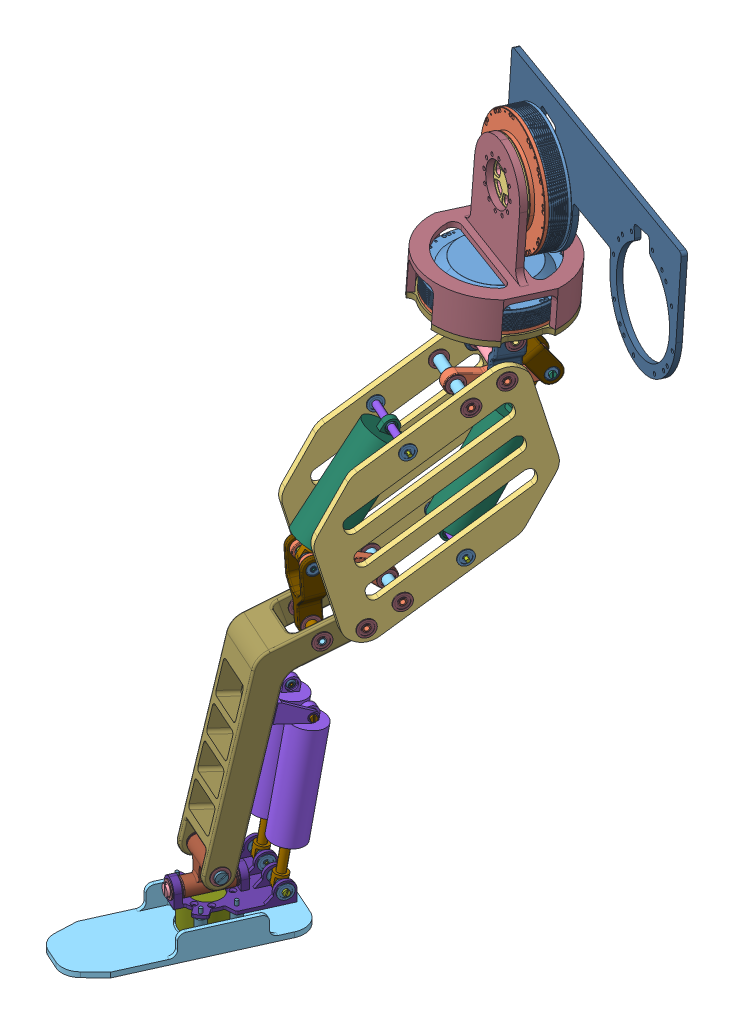
SolidWorks assembly 腿部总装, configuration 默认. Lengths in mm.
Overall size (628.66 1050.26 646.32).
180 component instances, 46 part files, 283 mates.
Components (placement in the parent):
- B1电机模型-220923.STEP-1: B1电机模型-220923.STEP [默认] at (664.8919 713.7763 -8377.8615) x (0.025023 0.998139 -0.055612) z (-0.344283 0.060831 0.936893) size (57.67 170.5 170.5)
  - B1________-220923.STEP.STEP-1: B1________-220923.STEP.STEP [默认] at origin size (57.67 170.5 170.5)
    - 11UXMR1_DVUR40_BCVR1_BASR1.STEP.STEP-1: 11UXMR1_DVUR40_BCVR1_BASR1.STEP.STEP [默认] at (17.5155 -7.1917 170.5) size (43.17 170.5 170.5)
    - 11UXMR1_DVUR40_HOSR1_BASR1.STEP.STEP-1: 11UXMR1_DVUR40_HOSR1_BASR1.STEP.STEP [默认] at (17.5155 -7.1917 170.5) size (28.4 170.5 170.5)
    - 11UXMR1_DVUR40_RDCR1_HLDR1_BHDR1.STEP.STEP-1: 11UXMR1_DVUR40_RDCR1_HLDR1_BHDR1.STEP.STEP [默认] at (17.5155 -7.1917 170.5) x (1 0 0) z (0 0.585761 -0.810484) size (4.4 117.7 117.7)
    - 11UXMR1_DVUR40_RDCR1_HLDR1_BASR1.STEP.STEP-1: 11UXMR1_DVUR40_RDCR1_HLDR1_BASR1.STEP.STEP [默认] at (17.5155 -7.1917 170.5) x (1 0 0) z (0 0.409019 0.912526) size (11.2 84 84)
- 脚掌-1: 脚掌 [默认] at (397.9595 0 -7737.8464) x (0.410325 0 -0.911939) z (0.911939 0 0.410325) size (300 40 105)
- 踝关节5mm轴套-1: 踝关节5mm轴套 [默认] at (545.6813 64 -7956.486) x (0.07714 0.98217 -0.171441) z (-0.911939 0 -0.410325) size (8 8 10.5)
- 踝关节5mm轴套-2: 踝关节5mm轴套 [默认] at (527.8985 64 -7964.4873) x (0.035137 0.996327 -0.078091) z (-0.911939 0 -0.410325) size (8 8 10.5)
- 脚踝推杆轴-1: 脚踝推杆轴 [默认] at (513.3075 64 -7971.0525) x (0.375312 -0.404204 -0.834122) z (0.911939 0 0.410325) size (13.49 9 44.5)
- 踝关节5mm轴套-3: 踝关节5mm轴套 [默认] at (473.1822 64 -7989.1068) x (0.07714 0.98217 -0.171441) z (-0.911939 0 -0.410325) size (8 8 10.5)
- 踝关节5mm轴套-4: 踝关节5mm轴套 [默认] at (490.965 64 -7981.1055) x (0.035137 0.996327 -0.078091) z (-0.911939 0 -0.410325) size (8 8 10.5)
- 脚踝推杆-1: 脚踝推杆 [默认] at (535.8997 123.2192 -7971.3029) x (-0.405206 0.158371 0.900404) z (-0.911913 -0.00001 -0.410384) size (50 247.76 50) (flexible)
  - 脚踝推杆本体-1: 脚踝推杆本体 [默认] at origin size (50 183.79 50)
  - 脚踝推杆伸缩杆-1: 脚踝推杆伸缩杆 [默认] at (0 -45.4761 0) x (-1 0 0) z (0 0 1) size (20 104.5 20)
  - 脚踝推杆球头-1: 脚踝推杆球头 [默认] at (-3.1478 -74.1303 0.0002) x (-0.976152 0.21709 0.000064) z (-0.000065 0 -1) size (13 13 9)
  - 脚踝推杆球头-2: 脚踝推杆球头 [默认] at (9.2552 155.5993 -0.0006) x (-0.769796 -0.63829 0.00005) z (-0.000065 0 -1) size (13 13 9)
- 脚踝交叉转轴套筒-1: 脚踝交叉转轴套筒 [默认] at (473.8697 64 -7906.5552) x (-0.911939 0 -0.410325) z (0.410325 0 -0.911939) size (55.5 60.31 62)
- 小腿骨-1: 小腿骨 [默认] at (444.0107 93.8936 -7941.9427) x (0.911939 0 0.410325) z (-0.400705 0.215269 0.890559) size (83.5 376.58 140.44)
- 法兰轴承10_22_6-6: 法兰轴承10_22_6 [默认] at (440.8119 98.3066 -7921.4295) x (0.009593 0.999727 -0.02132) z (0.410213 -0.023378 -0.91169) size (25 6 25)
- 法兰轴承10_22_6-7: 法兰轴承10_22_6 [默认] at (439.8999 98.3066 -7921.8398) x (-0.044167 0.99419 0.09816) z (-0.407941 -0.107639 0.906641) size (25 6 25)
- 法兰轴承10_22_6-8: 法兰轴承10_22_6 [默认] at (506.9275 98.3066 -7891.6809) x (-0.044167 0.99419 0.09816) z (-0.407941 -0.107639 0.906641) size (25 6 25)
- 法兰轴承10_22_6-9: 法兰轴承10_22_6 [默认] at (507.8394 98.3066 -7891.2706) x (0.009593 0.999727 -0.02132) z (0.410213 -0.023378 -0.91169) size (25 6 25)
- 直径10轴-1: 直径10轴 [默认] at (434.8843 98.3066 -7924.0966) x (0.245458 -0.801344 -0.545526) z (0.911939 0 0.410325) size (16.99 16 90)
- 脚踝推杆-4: 脚踝推杆 [默认] at (481.1834 123.2192 -7995.9224) x (0.409589 -0.158369 -0.898419) z (0.909953 0.000772 0.414711) size (50 247.76 50) (flexible)
  - 脚踝推杆本体-1: 脚踝推杆本体 [默认] at origin size (50 183.79 50)
  - 脚踝推杆伸缩杆-1: 脚踝推杆伸缩杆 [默认] at (0 -45.4761 0) x (-1 0 0) z (0 0 1) size (20 104.5 20)
  - 脚踝推杆球头-1: 脚踝推杆球头 [默认] at (4.0411 -73.9016 -0.0197) x (0.960367 0.278701 -0.004683) z (0.004877 0 0.999988) size (13 13 9)
  - 脚踝推杆球头-2: 脚踝推杆球头 [默认] at (1.7961 152.373 -0.0088) x (0.992287 0.12387 -0.004839) z (0.004877 0 0.999988) size (13 13 9)
- 膝髋推杆-1: 膝髋推杆 [默认] at (526.5494 496.4932 -8023.6348) x (0.342168 -0.551924 -0.760461) z (0.911939 0 0.410325) size (65 205.29 65) (flexible)
  - 膝髋推杆本体-1: 膝髋推杆本体 [默认] at origin size (65 180.79 65)
  - 脚踝推杆球头-1: 脚踝推杆球头 [默认] at (-4.3874 149.941 0) x (0.953124 -0.30258 0) z (0 0 1) size (13 13 9)
  - 脚踝推杆伸缩杆-1: 脚踝推杆伸缩杆 [默认] at (0 -6 0) x (-1 0 0) z (0 0 1) size (20 104.5 20)
  - 脚踝推杆球头-2: 脚踝推杆球头 [默认] at (-4.4262 -34.3079 0) x (0.95227 -0.305256 0) z (0 0 1) size (13 13 9)
- 法兰轴承10_22_6-10: 法兰轴承10_22_6 [默认] at (509.3879 404.6089 -8076.2753) x (-0.155995 -0.924915 0.346696) z (0.379516 -0.380175 -0.843466) size (25 6 25)
- 法兰轴承10_22_6-11: 法兰轴承10_22_6 [默认] at (510.2998 404.6089 -8075.865) x (0.133117 0.945914 -0.295849) z (0.388132 -0.324418 -0.862616) size (25 6 25)
- 法兰轴承10_22_6-12: 法兰轴承10_22_6 [默认] at (576.4154 404.6089 -8046.1164) x (-0.203068 0.868952 0.451315) z (-0.356553 -0.494896 0.792432) size (25 6 25)
- 法兰轴承10_22_6-13: 法兰轴承10_22_6 [默认] at (577.3273 404.6089 -8045.7061) x (0.410254 0.018565 -0.911782) z (0.007617 -0.999828 -0.01693) size (25 6 25)
- 六轴力_力矩传感器-1: 六轴力_力矩传感器 [默认] at (473.8697 8 -7906.5552) x (0.911939 0 0.410325) z (0 1 0) size (92 76.2 38)
- 六轴力_力矩传感器安装板-1: 六轴力_力矩传感器安装板 [默认] at (473.8697 13 -7906.5552) x (0.811322 0 -0.5846) z (0 1 0) size (148.3 135.37 35)
- 膝关节U型架-1: 膝关节U型架 [默认] at (524.2631 388.7482 -8000.8845) x (-0.911939 0 -0.410325) z (0.409787 0.05122 -0.910742) size (56 120 30)
- 轴承_NSK635-10: 轴承_NSK635 [默认] at (501.8441 479.3983 -8022.3438) x (0.003655 -0.99996 -0.008124) z (0.410309 0.008909 -0.911903) size (19 6 19)
- 轴承_NSK635-11: 轴承_NSK635 [默认] at (547.4411 479.3983 -8001.8276) x (-0.094561 -0.973083 0.21016) z (0.399281 -0.230453 -0.887393) size (19 6 19)
- 膝关节U型架后侧-1: 膝关节U型架后侧 [默认] at (560.8965 434.6133 -8082.3016) x (-0.911939 0 -0.410325) z (0.155672 0.925238 -0.345978) size (38 132.57 35.17)
- 法兰轴承10_22_6-15: 法兰轴承10_22_6 [默认] at (563.5672 429.8849 -8099.204) x (0.123874 0.953342 -0.275308) z (0.39118 -0.301893 -0.86939) size (25 6 25)
- 法兰轴承10_22_6-16: 法兰轴承10_22_6 [默认] at (558.5515 429.8849 -8101.4608) x (-0.212239 0.855836 0.471698) z (-0.351171 -0.517247 0.780471) size (25 6 25)
- 大腿侧板-1: 大腿侧板 [默认] at (445.6606 446.5602 -7979.729) x (0.356655 -0.494461 -0.792658) z (0.911939 0 0.410325) size (240 380 10)
- 法兰轴承10_22_6-17: 法兰轴承10_22_6 [默认] at (496.6207 404.6089 -8082.0198) x (0.03518 0.996318 -0.078187) z (-0.408814 0.085737 0.908581) size (25 6 25)
- 法兰轴承10_22_6-18: 法兰轴承10_22_6 [默认] at (497.5327 404.6089 -8081.6095) x (0.384602 0.348494 -0.854771) z (0.142996 -0.937311 -0.317806) size (25 6 25)
- 法兰轴承10_22_6-19: 法兰轴承10_22_6 [默认] at (514.3225 429.8849 -8121.3616) x (-0.147464 0.93319 0.327737) z (-0.382911 -0.359384 0.851012) size (25 6 25)
- 法兰轴承10_22_6-20: 法兰轴承10_22_6 [默认] at (515.2344 429.8849 -8120.9513) x (0.104625 0.966946 -0.232526) z (0.396762 -0.25498 -0.881796) size (25 6 25)
- 膝关节10mm轴套-1: 膝关节10mm轴套 [默认] at (569.1199 404.6089 -8049.399) x (0.165501 -0.915049 -0.367823) z (-0.911939 0 -0.410325) size (15 15 58.5)
- 轴承_NSK635-13: 轴承_NSK635 [默认] at (510.0516 479.3983 -8018.6509) x (-0.094561 -0.973083 0.21016) z (0.399281 -0.230453 -0.887393) size (19 6 19)
- 轴承_NSK635-14: 轴承_NSK635 [默认] at (539.2336 479.3983 -8005.5205) x (-0.089688 -0.975819 0.19933) z (0.400403 -0.218578 -0.889888) size (19 6 19)
- 膝关节10mm轴套2-1: 膝关节10mm轴套2 [默认] at (553.0799 429.8849 -8103.9228) x (0.319809 -0.626521 -0.710769) z (-0.911939 0 -0.410325) size (15 15 35.5)
- 膝关节5mm轴套2-3: 膝关节5mm轴套2 [默认] at (541.9695 479.3983 -8004.2895) x (0.366223 -0.45101 -0.813923) z (-0.911939 0 -0.410325) size (10 10 3)
- 膝关节5mm轴套3-2: 膝关节5mm轴套3 [默认] at (533.762 479.3983 -8007.9824) x (0.22509 -0.836108 -0.500258) z (-0.911939 0 -0.410325) size (10 10 8.5)
- 膝关节5mm轴套3-3: 膝关节5mm轴套3 [默认] at (517.8031 479.3983 -8015.1631) x (0.22509 -0.836108 -0.500258) z (-0.911939 0 -0.410325) size (10 10 8.5)
- 膝关节10mm轴套2-2: 膝关节10mm轴套2 [默认] at (601.4127 429.8849 -8082.1755) x (0.319809 -0.626521 -0.710769) z (-0.911939 0 -0.410325) size (15 15 35.5)
- 大腿侧板-2: 大腿侧板 [默认] at (538.2225 446.5602 -7938.081) x (0.356655 -0.494461 -0.792658) z (0.911939 0 0.410325) size (240 380 10)
- 法兰轴承10_22_6-21: 法兰轴承10_22_6 [默认] at (606.8843 429.8849 -8079.7136) x (0.104625 0.966946 -0.232526) z (-0.396762 0.25498 0.881796) size (25 6 25)
- 法兰轴承10_22_6-22: 法兰轴承10_22_6 [默认] at (589.1826 404.6089 -8040.3718) x (0.384602 0.348494 -0.854771) z (-0.142996 0.937311 0.317806) size (25 6 25)
- 法兰轴承10_22_6-23: 法兰轴承10_22_6 [默认] at (590.0945 404.6089 -8039.9615) x (0.03518 0.996318 -0.078187) z (0.408814 -0.085737 -0.908581) size (25 6 25)
- 法兰轴承10_22_6-24: 法兰轴承10_22_6 [默认] at (607.7962 429.8849 -8079.3033) x (-0.147464 0.93319 0.327737) z (0.382911 0.359384 -0.851012) size (25 6 25)
- 膝髋推杆-2: 膝髋推杆 [默认] at (624.78 614.7303 -8241.9502) x (-0.391704 0.486585 0.780899) z (0.898137 0.017912 0.43935) size (65 254.69 65) (flexible)
  - 膝髋推杆本体-1: 膝髋推杆本体 [默认] at origin size (65 180.79 65)
  - 脚踝推杆球头-1: 脚踝推杆球头 [默认] at (-8.7962 152.2386 -0.3238) x (0.79413 -0.607044 0.029234) z (-0.036788 0 0.999323) size (13 13 9)
  - 脚踝推杆伸缩杆-1: 脚踝推杆伸缩杆 [默认] at (0 -55.4056 0) x (-1 0 0) z (0 0 1) size (20 104.5 20)
  - 脚踝推杆球头-2: 脚踝推杆球头 [默认] at (-8.7962 -81.4283 -0.3238) x (0.79413 -0.607044 0.029234) z (-0.036788 0 0.999323) size (13 13 9)
- 膝关节5mm轴套4-1: 膝关节5mm轴套4 [默认] at (559.5325 633.0528 -8107.9058) x (0.165546 -0.915001 -0.367922) z (-0.911939 0 -0.410325) size (10 10 39.75)
- 膝关节5mm轴套4-2: 膝关节5mm轴套4 [默认] at (603.9895 633.0528 -8087.9025) x (0.165546 -0.915001 -0.367922) z (-0.911939 0 -0.410325) size (10 10 39.75)
- 膝关节U型架后侧-2: 膝关节U型架后侧 [默认] at (608.1443 678.4135 -8187.3088) x (-0.911939 0 -0.410325) z (0.040214 -0.995186 -0.089374) size (38 132.57 35.17)
- 轴承_NSK635-19: 轴承_NSK635 [默认] at (656.0735 675.7893 -8265.1947) x (-0.089688 -0.975819 0.19933) z (0.400403 -0.218578 -0.889888) size (19 6 19)
- 轴承_NSK635-20: 轴承_NSK635 [默认] at (626.8915 675.7893 -8278.3251) x (-0.089688 -0.975819 0.19933) z (0.400403 -0.218578 -0.889888) size (19 6 19)
- 法兰轴承10_22_6-26: 法兰轴承10_22_6 [默认] at (592.1305 674.861 -8176.0895) x (-0.161282 0.919513 0.358446) z (-0.377299 -0.393059 0.83854) size (25 6 25)
- 法兰轴承10_22_6-27: 法兰轴承10_22_6 [默认] at (597.1462 674.861 -8173.8327) x (0.123937 0.953293 -0.275448) z (0.39116 -0.302046 -0.869346) size (25 6 25)
- 膝关节5mm轴套4-3: 膝关节5mm轴套4 [默认] at (587.9578 471.6931 -8171.0806) x (0.174936 -0.904565 -0.388792) z (-0.911939 0 -0.410325) size (10 10 39.75)
- 法兰轴承10_22_6-28: 法兰轴承10_22_6 [默认] at (547.9015 674.861 -8195.9902) x (0.21516 0.851493 -0.478189) z (-0.349389 0.524365 0.77651) size (25 6 25)
- 法兰轴承10_22_6-29: 法兰轴承10_22_6 [默认] at (565.6032 700.1369 -8235.332) x (0.21516 0.851493 -0.478189) z (-0.349389 0.524365 0.77651) size (25 6 25)
- 法兰轴承10_22_6-30: 法兰轴承10_22_6 [默认] at (566.5152 700.1369 -8234.9217) x (-0.380944 -0.371597 0.846639) z (-0.152475 0.928394 0.338874) size (25 6 25)
- 法兰轴承10_22_6-31: 法兰轴承10_22_6 [默认] at (548.8134 674.861 -8195.5799) x (0.380944 0.371597 -0.846639) z (0.152475 -0.928394 -0.338874) size (25 6 25)
- 膝关节10mm轴套2-3: 膝关节10mm轴套2 [默认] at (586.6589 674.861 -8178.5514) x (0.165521 -0.915028 -0.367868) z (-0.911939 0 -0.410325) size (15 15 35.5)
- 膝关节U型架-2: 膝关节U型架 [默认] at (628.7298 757.5372 -8233.0597) x (-0.911939 0 -0.410325) z (-0.332668 -0.585402 0.739349) size (56 120 30)
- 法兰轴承10_22_6-32: 法兰轴承10_22_6 [默认] at (490.7405 389.5165 -8032.3948) x (0.21516 0.851493 -0.478189) z (0.349389 -0.524365 -0.77651) size (25 6 25)
- 法兰轴承10_22_6-33: 法兰轴承10_22_6 [默认] at (489.8286 389.5165 -8032.8052) x (-0.381375 -0.368959 0.847598) z (0.151393 -0.929446 -0.336468) size (25 6 25)
- 法兰轴承10_22_6-34: 法兰轴承10_22_6 [默认] at (521.2905 389.5165 -8018.6489) x (-0.381368 -0.369 0.847583) z (0.15141 -0.929429 -0.336506) size (25 6 25)
- 法兰轴承10_22_6-35: 法兰轴承10_22_6 [默认] at (556.8561 389.5165 -8002.6463) x (0.21516 0.851493 -0.478189) z (-0.349389 0.524365 0.77651) size (25 6 25)
- 法兰轴承10_22_6-36: 法兰轴承10_22_6 [默认] at (557.7681 389.5165 -8002.2359) x (-0.381375 -0.368959 0.847598) z (-0.151393 0.929446 0.336468) size (25 6 25)
- 法兰轴承10_22_6-37: 法兰轴承10_22_6 [默认] at (526.3062 389.5165 -8016.3921) x (-0.381368 -0.369 0.847583) z (-0.15141 0.929429 0.336506) size (25 6 25)
- 膝关节10mm轴套3-1: 膝关节10mm轴套3 [默认] at (515.8188 389.5165 -8021.1109) x (0.409301 -0.07062 -0.909662) z (-0.911939 0 -0.410325) size (15 15 21.5)
- 膝关节10mm轴套3-2: 膝关节10mm轴套3 [默认] at (551.3845 389.5165 -8005.1082) x (0.409301 -0.07062 -0.909662) z (-0.911939 0 -0.410325) size (15 15 21.5)
- 法兰轴承10_22_6-38: 法兰轴承10_22_6 [默认] at (614.6204 748.7562 -8226.0727) x (0.215153 0.851505 -0.478172) z (-0.349394 0.524346 0.776521) size (25 6 25)
- 法兰轴承10_22_6-39: 法兰轴承10_22_6 [默认] at (619.636 748.7562 -8223.8159) x (-0.380939 -0.371622 0.84663) z (-0.152486 0.928384 0.338896) size (25 6 25)
- 法兰轴承10_22_6-40: 法兰轴承10_22_6 [默认] at (658.165 700.1369 -8193.684) x (-0.380944 -0.371597 0.846639) z (0.152475 -0.928394 -0.338874) size (25 6 25)
- 法兰轴承10_22_6-41: 法兰轴承10_22_6 [默认] at (640.4633 674.861 -8154.3422) x (0.380944 0.371597 -0.846639) z (-0.152475 0.928394 0.338874) size (25 6 25)
- 法兰轴承10_22_6-42: 法兰轴承10_22_6 [默认] at (659.077 700.1369 -8193.2737) x (0.21516 0.851493 -0.478189) z (0.349389 -0.524365 -0.77651) size (25 6 25)
- 法兰轴承10_22_6-43: 法兰轴承10_22_6 [默认] at (641.3752 674.861 -8153.9319) x (0.21516 0.851493 -0.478189) z (0.349389 -0.524365 -0.77651) size (25 6 25)
- 膝关节10mm轴套2-4: 膝关节10mm轴套2 [默认] at (634.9917 674.861 -8156.8042) x (0.165521 -0.915028 -0.367868) z (-0.911939 0 -0.410325) size (15 15 35.5)
- 膝关节5mm轴套4-4: 膝关节5mm轴套4 [默认] at (632.4148 471.6931 -8151.0772) x (0.174936 -0.904565 -0.388792) z (-0.911939 0 -0.410325) size (10 10 39.75)
- 膝关节5mm轴套3-4: 膝关节5mm轴套3 [默认] at (634.6429 675.7893 -8274.8373) x (0.22844 -0.830695 -0.507702) z (-0.911939 0 -0.410325) size (10 10 8.5)
- 膝关节5mm轴套2-5: 膝关节5mm轴套2 [默认] at (621.4198 675.7893 -8280.7871) x (0.366223 -0.45101 -0.813923) z (-0.911939 0 -0.410325) size (10 10 3)
- 轴承_NSK635-28: 轴承_NSK635 [默认] at (613.2124 675.7893 -8284.48) x (-0.094561 -0.973083 0.21016) z (-0.399281 0.230453 0.887393) size (19 6 19)
- 膝关节5mm轴套3-5: 膝关节5mm轴套3 [默认] at (650.6019 675.7893 -8267.6567) x (0.22844 -0.830695 -0.507702) z (-0.911939 0 -0.410325) size (10 10 8.5)
- 膝关节5mm轴套2-6: 膝关节5mm轴套2 [默认] at (658.8093 675.7893 -8263.9637) x (0.366223 -0.45101 -0.813923) z (-0.911939 0 -0.410325) size (10 10 3)
- 轴承_NSK635-29: 轴承_NSK635 [默认] at (664.281 675.7893 -8261.5018) x (-0.094561 -0.973083 0.21016) z (0.399281 -0.230453 -0.887393) size (19 6 19)
- 髋关节座-1: 髋关节座 [默认] at (614.1978 774.2391 -8218.4315) x (0.409561 -0.060982 -0.910242) z (-0.025023 -0.998139 0.055612) size (84 125 90)
- 法兰轴承10_22_6-44: 法兰轴承10_22_6 [默认] at (574.0391 748.7562 -8244.3322) x (-0.147473 0.933182 0.327756) z (-0.382908 -0.359405 0.851005) size (25 6 25)
- 法兰轴承10_22_6-46: 法兰轴承10_22_6 [默认] at (575.8629 748.7562 -8243.5115) x (-0.380947 -0.371576 0.846647) z (-0.152467 0.928403 0.338855) size (25 6 25)
- 法兰轴承10_22_6-47: 法兰轴承10_22_6 [默认] at (580.1942 700.1369 -8228.7668) x (0.389203 0.316708 -0.864995) z (0.129953 -0.948523 -0.288819) size (25 6 25)
- 法兰轴承10_22_6-48: 法兰轴承10_22_6 [默认] at (644.486 700.1369 -8199.8389) x (0.389203 0.316708 -0.864995) z (-0.129953 0.948523 0.288819) size (25 6 25)
- 法兰轴承10_22_6-50: 法兰轴承10_22_6 [默认] at (658.3935 748.7562 -8206.3771) x (-0.380947 -0.371576 0.846647) z (0.152467 -0.928403 -0.338855) size (25 6 25)
- 法兰轴承10_22_6-51: 法兰轴承10_22_6 [默认] at (660.2173 748.7562 -8205.5564) x (-0.147473 0.933182 0.327756) z (0.382908 0.359405 -0.851005) size (25 6 25)
- 膝关节10mm轴套-3: 膝关节10mm轴套 [默认] at (639.0143 700.1369 -8202.3008) x (0.165501 -0.915049 -0.367823) z (-0.911939 0 -0.410325) size (15 15 58.5)
- 膝关节5mm轴套2-7: 膝关节5mm轴套2 [默认] at (504.5799 479.3983 -8021.1128) x (0.366223 -0.45101 -0.813923) z (-0.911939 0 -0.410325) size (10 10 3)
- 髋关节10mm轴套-1: 髋关节10mm轴套 [默认] at (609.1487 748.7562 -8228.5346) x (0.165546 -0.915001 -0.367922) z (-0.911939 0 -0.410325) size (15 15 30.5)
- 髋关节10mm轴套-2: 髋关节10mm轴套 [默认] at (652.9218 748.7562 -8208.839) x (0.165546 -0.915001 -0.367922) z (-0.911939 0 -0.410325) size (15 15 30.5)
- B1电机模型-220923-1: B1电机模型-220923 [默认] at (445.6066 963.7855 -8243.8963) x (0.344283 -0.060831 -0.936893) z (0.925879 -0.143408 0.349547) size (57.67 170.5 170.5)
  - B1电机模型-220923.STEP-1: B1电机模型-220923.STEP [默认] at origin size (57.67 170.5 170.5)
    - B1________-220923.STEP.STEP-1: B1________-220923.STEP.STEP [默认] at origin size (57.67 170.5 170.5)
      - 11UXMR1_DVUR40_BCVR1_BASR1.STEP.STEP-1: 11UXMR1_DVUR40_BCVR1_BASR1.STEP.STEP [默认] at (17.5155 -7.1917 170.5) size (43.17 170.5 170.5)
      - 11UXMR1_DVUR40_HOSR1_BASR1.STEP.STEP-1: 11UXMR1_DVUR40_HOSR1_BASR1.STEP.STEP [默认] at (17.5155 -7.1917 170.5) size (28.4 170.5 170.5)
      - 11UXMR1_DVUR40_RDCR1_HLDR1_BHDR1.STEP.STEP-1: 11UXMR1_DVUR40_RDCR1_HLDR1_BHDR1.STEP.STEP [默认] at (17.5155 -7.1917 170.5) x (1 0 0) z (0 0.585761 -0.810484) size (4.4 117.7 117.7)
      - 11UXMR1_DVUR40_RDCR1_HLDR1_BASR1.STEP.STEP-1: 11UXMR1_DVUR40_RDCR1_HLDR1_BASR1.STEP.STEP [默认] at (17.5155 -7.1917 170.5) x (1 0 0) z (0 0.409019 0.912526) size (11.2 84 84)
- 髋关节电机固定座-1: 髋关节电机固定座 [默认] at (614.2353 775.7364 -8218.5149) x (-0.485242 0.060764 0.872266) z (0.025023 0.998139 -0.055612) size (192.33 192.33 8)
- 髋关节电机固定座2-1: 髋关节电机固定座2 [默认] at (615.6366 831.6321 -8221.6292) x (0.874022 0.005159 0.485859) z (0.025023 0.998139 -0.055612) size (192.33 196 206)
- 法兰轴承10_22_6-52: 法兰轴承10_22_6 [默认] at (457.2515 64 -7869.6216) x (0.031977 0.999385 0.014388) z (0.911378 -0.035064 0.410073) size (25 6 25)
- 法兰轴承10_22_6-53: 法兰轴承10_22_6 [默认] at (457.6618 64 -7870.5336) x (0.427699 0.883199 0.192442) z (-0.805424 0.468999 -0.362399) size (25 6 25)
- 法兰轴承10_22_6-54: 法兰轴承10_22_6 [默认] at (490.0775 64 -7942.5768) x (0.031977 0.999385 0.014388) z (0.911378 -0.035064 0.410073) size (25 6 25)
- 法兰轴承10_22_6-55: 法兰轴承10_22_6 [默认] at (490.4879 64 -7943.4887) x (0.427449 0.883344 0.19233) z (-0.805556 0.468725 -0.362458) size (25 6 25)
- 橡胶减震套-1: 橡胶减震套 [默认] at (516.6515 46 -7910.8817) x (1 0 0) z (0 -1 0) size (15 15 42)
- 橡胶减震套-2: 橡胶减震套 [默认] at (448.7319 46 -7941.442) x (1 0 0) z (0 -1 0) size (15 15 42)
- 橡胶减震套-3: 橡胶减震套 [默认] at (431.0879 46 -7902.2286) x (1 0 0) z (0 -1 0) size (15 15 42)
- 橡胶减震套-4: 橡胶减震套 [默认] at (499.0075 46 -7871.6683) x (1 0 0) z (0 -1 0) size (15 15 42)
- 脚掌5mm轴套-1: 脚掌5mm轴套 [默认] at (516.6515 8 -7910.8817) x (0.992254 0 0.124222) z (0 1 0) size (15 15 8)
- 法兰轴承10_22_6-56: 法兰轴承10_22_6 [默认] at (646.3098 700.1369 -8199.0182) x (0.21516 0.851493 -0.478189) z (0.349389 -0.524365 -0.77651) size (25 6 25)
- 法兰轴承10_22_6-57: 法兰轴承10_22_6 [默认] at (578.3704 700.1369 -8229.5874) x (0.21516 0.851493 -0.478189) z (-0.349389 0.524365 0.77651) size (25 6 25)
- 膝关节10mm轴套4-1: 膝关节10mm轴套4 [默认] at (503.0043 404.6089 -8079.1476) x (0.388891 -0.318978 -0.864302) z (0.911939 0 0.410325) size (15 15 1)
- 膝关节10mm轴套4-2: 膝关节10mm轴套4 [默认] at (571.9868 700.1369 -8232.4597) x (0.388891 -0.318978 -0.864302) z (0.911939 0 0.410325) size (15 15 1)
- 膝关节10mm轴套4-3: 膝关节10mm轴套4 [默认] at (651.7815 700.1369 -8196.5563) x (0.388891 -0.318978 -0.864302) z (0.911939 0 0.410325) size (15 15 1)
- 膝关节10mm轴套4-4: 膝关节10mm轴套4 [默认] at (582.799 404.6089 -8043.2441) x (0.388891 -0.318978 -0.864302) z (0.911939 0 0.410325) size (15 15 1)
- 法兰轴承10_22_6-58: 法兰轴承10_22_6 [默认] at (495.0723 98.3066 -7897.0151) x (0.218862 -0.845872 -0.486416) z (-0.347083 -0.533386 0.771384) size (25 6 25)
- 膝关节10mm轴套4-5: 膝关节10mm轴套4 [默认] at (500.5439 98.3066 -7894.5532) x (-0.212581 -0.855332 0.472458) z (0.911939 0 0.410325) size (15 15 1)
- 膝关节10mm轴套4-6: 膝关节10mm轴套4 [默认] at (446.2835 98.3066 -7918.9675) x (-0.212581 -0.855332 0.472458) z (0.911939 0 0.410325) size (15 15 1)
- 法兰轴承10_22_6-59: 法兰轴承10_22_6 [默认] at (452.6671 98.3066 -7916.0952) x (0.218862 -0.845872 -0.486416) z (0.347083 0.533386 -0.771384) size (25 6 25)
- 法兰轴承10_22_6-60: 法兰轴承10_22_6 [默认] at (484.7433 64 -7930.7216) x (-0.358203 0.919627 -0.161173) z (-0.838644 -0.392792 -0.377346) size (25 6 25)
- 膝关节10mm轴套4-7: 膝关节10mm轴套4 [默认] at (487.2053 64 -7936.1932) x (0.472861 -0.855064 0.212763) z (0.410325 0 -0.911939) size (15 15 1)
- 法兰轴承10_22_6-61: 法兰轴承10_22_6 [默认] at (462.9961 64 -7882.3888) x (0.020099 0.999757 0.009044) z (0.911718 -0.02204 0.410226) size (25 6 25)
- 膝关节10mm轴套4-8: 膝关节10mm轴套4 [默认] at (460.1238 64 -7876.0052) x (0.472861 -0.855064 0.212763) z (0.410325 0 -0.911939) size (15 15 1)
- 法兰轴承5_11_5-1: 法兰轴承5_11_5 [默认] at (553.804 287.8759 -7992.2073) x (-0.26289 -0.767802 0.584268) z (-0.315049 0.640687 0.700189) size (12.5 5 12.5)
- 膝关节5mm轴套5-1: 膝关节5mm轴套5 [默认] at (550.8402 287.8759 -7993.5409) x (0.410325 0.000604 -0.911939) z (0.911939 0 0.410325) size (8 8 3.25)
- 膝关节5mm轴套5-2: 膝关节5mm轴套5 [默认] at (484.9526 287.8759 -8023.1869) x (0.410325 0.000604 -0.911939) z (0.911939 0 0.410325) size (8 8 3.25)
- 法兰轴承5-19-6-1: 法兰轴承5-19-6 [默认] at (545.3246 471.6931 -8190.2633) x (0.409328 -0.069689 -0.909722) z (0.028595 0.997569 -0.063552) size (22 6 22)
- 法兰轴承5-19-6-2: 法兰轴承5-19-6 [默认] at (516.8993 633.0528 -8127.0885) x (0.409328 -0.069689 -0.909722) z (0.028595 0.997569 -0.063552) size (22 6 22)
- 法兰轴承5-19-6-3: 法兰轴承5-19-6 [默认] at (517.8112 633.0528 -8126.6782) x (-0.168367 0.911939 0.374192) z (0.374192 0.410325 -0.831633) size (22 6 22)
- 法兰轴承5-19-6-4: 法兰轴承5-19-6 [默认] at (546.2366 471.6931 -8189.853) x (0.168367 -0.911939 -0.374192) z (-0.374192 -0.410325 0.831633) size (22 6 22)
- 法兰轴承5-19-6-5: 法兰轴承5-19-6 [默认] at (638.7984 471.6931 -8148.205) x (0.409328 -0.069689 -0.909722) z (-0.028595 -0.997569 0.063552) size (22 6 22)
- 法兰轴承5-19-6-6: 法兰轴承5-19-6 [默认] at (637.8865 471.6931 -8148.6153) x (0.168367 -0.911939 -0.374192) z (0.374192 0.410325 -0.831633) size (22 6 22)
- 法兰轴承5-19-6-7: 法兰轴承5-19-6 [默认] at (610.3731 633.0528 -8085.0302) x (0.409328 -0.069689 -0.909722) z (-0.028595 -0.997569 0.063552) size (22 6 22)
- 法兰轴承5-19-6-8: 法兰轴承5-19-6 [默认] at (609.4611 633.0528 -8085.4405) x (-0.168367 0.911939 0.374192) z (-0.374192 -0.410325 0.831633) size (22 6 22)
- 法兰轴承5-19-6-9: 法兰轴承5-19-6 [默认] at (545.6813 64 -7956.486) x (-0.292893 -0.700341 0.65095) z (-0.287368 0.713808 0.638669) size (22 6 22)
- 法兰轴承5-19-6-10: 法兰轴承5-19-6 [默认] at (518.3232 64 -7968.7957) x (0.409328 -0.069689 -0.909722) z (0.028595 0.997569 -0.063552) size (22 6 22)
- 法兰轴承5-19-6-12: 法兰轴承5-19-6 [默认] at (463.6068 64 -7993.4153) x (-0.292893 -0.700341 0.65095) z (0.287368 -0.713808 -0.638669) size (22 6 22)
- 法兰轴承5-19-6-13: 法兰轴承5-19-6 [默认] at (490.965 64 -7981.1055) x (0.409328 -0.069689 -0.909722) z (-0.028595 -0.997569 0.063552) size (22 6 22)
- 脚踝推杆轴-3: 脚踝推杆轴 [默认] at (495.9806 64 -7978.8487) x (-0.375312 0.404204 0.834122) z (-0.911939 0 -0.410325) size (13.49 9 44.5)
- 法兰轴承5_11_5-2: 法兰轴承5_11_5 [默认] at (484.9526 287.8759 -8023.1869) x (-0.26289 -0.767802 0.584268) z (0.315049 -0.640687 -0.700189) size (12.5 5 12.5)
- 直径10轴2-1: 直径10轴2 [默认] at (646.3909 674.861 -8151.6751) x (0.14188 -0.938317 -0.315326) z (-0.911939 0 -0.410325) size (16.99 16 118)
- 直径10轴2-2: 直径10轴2 [默认] at (612.8119 429.8849 -8077.0465) x (0.14188 -0.938317 -0.315326) z (-0.911939 0 -0.410325) size (16.99 16 118)
- 直径10轴2-3: 直径10轴2 [默认] at (595.1102 404.6089 -8037.7047) x (0.14188 -0.938317 -0.315326) z (-0.911939 0 -0.410325) size (16.99 16 118)
- 直径10轴2-4: 直径10轴2 [默认] at (664.0927 700.1369 -8191.0169) x (0.14188 -0.938317 -0.315326) z (-0.911939 0 -0.410325) size (16.99 16 118)
- 直径10轴3-1: 直径10轴3 [默认] at (665.233 748.7562 -8203.2996) x (0.14188 -0.938317 -0.315326) z (-0.911939 0 -0.410325) size (16.99 16 110)
- 直径10轴4-1: 直径10轴4 [默认] at (492.7446 64 -7948.5044) x (0.911939 0 0.410325) z (-0.410325 0 0.911939) size (16.99 16 96.5)
- 直径10轴5-1: 直径10轴5 [默认] at (562.7837 389.5165 -7999.9791) x (0.14188 -0.938317 -0.315326) z (-0.911939 0 -0.410325) size (16.99 16 90)
- 5mm轴1-1: 5mm轴1 [默认] at (546.9851 479.3983 -8002.0327) x (0.14188 -0.938317 -0.315326) z (-0.911939 0 -0.410325) size (13.49 9 58.5)
- 5mm轴1-2: 5mm轴1 [默认] at (613.6683 675.7893 -8284.2748) x (0.410325 0 -0.911939) z (0.911939 0 0.410325) size (13.49 9 58.5)
- 5mm轴2-1: 5mm轴2 [默认] at (650.1977 471.6931 -8143.0759) x (0.14188 -0.938317 -0.315326) z (-0.911939 0 -0.410325) size (9 9 124)
- 5mm轴2-2: 5mm轴2 [默认] at (621.7723 633.0528 -8079.9011) x (0.14188 -0.938317 -0.315326) z (-0.911939 0 -0.410325) size (9 9 124)
- 脚踝推杆上固定座-1: 脚踝推杆上固定座 [默认] at (501.0751 303.8529 -7967.0187) x (-0.911939 0 -0.410325) z (0.400705 -0.215269 -0.890559) size (83.5 28 55)
- 5mm轴3-1: 5mm轴3 [默认] at (543.0887 287.8759 -7997.0287) x (0.410325 0 -0.911939) z (0.911939 0 0.410325) size (13.49 9 19.75)
- 5mm轴3-2: 5mm轴3 [默认] at (495.6679 287.8759 -8018.3656) x (-0.410325 0 0.911939) z (-0.911939 0 -0.410325) size (13.49 9 19.75)
- 腰部固定板-3: 腰部固定板 [默认] at (895.2986 929.0593 -8184.2115) x (0.938804 0.010813 0.344283) z (-0.344283 0.060831 0.936893) size (450 207.5 8)
Mates (geometry in assembly coordinates):
- 同心1: concentric anti-aligned: cylinder of 踝关节腕关节线性执行器A-81138 SEA801-189^腿部总装-1 through (-87.6589 77.3567 157.5565) axis (0 1 0) radius 2.5; cylinder of 脚掌-1 through (-191.7001 117.5768 210.1209) axis (0.002571 -0.999927 -0.011812) radius 8
- 同心4: concentric anti-aligned: cylinder of 轴承_NSK635-1 through (545.0759 64 -8043.1468) axis (-0.911939 0 -0.410325) radius 2.5; cylinder of 踝关节5mm轴套-1 through (580.7897 64 -8060.1031) axis (0.911939 0 0.410325) radius 2.6
- 同心5: concentric anti-aligned: cylinder of 轴承_NSK635-2 through (580.6415 64 -8027.1442) axis (-0.911939 0 -0.410325) radius 2.5; cylinder of 踝关节5mm轴套-2 through (563.0069 64 -8068.1044) axis (0.911939 0 0.410325) radius 2.6
- 重合5: coincident anti-aligned: plane of 踝关节腕关节线性执行器A-81138 SEA801-189^腿部总装-1 through (-86.1992 96.3567 153.8323) normal (0 -1 0); plane of 踝关节5mm轴套-1 through (580.7897 64 -8060.1031) normal (-0.911939 0 -0.410325)
- 重合6: coincident aligned: circle of 脚掌-1; circle of 轴承_NSK6900NR-1
- 重合71: coincident anti-aligned: plane of 脚掌-1 through (490.5201 8 -7815.613) normal (0 1 0); plane of 轴承_NSK6900NR-2 through (-348.0536 -237.1058 127.5565) normal (0 0 -1)
- 重合8: coincident anti-aligned: circle of 脚掌-1; circle of 轴承_NSK6900NR-3
- 重合9: coincident anti-aligned: circle of 脚掌-1; circle of 轴承_NSK6900NR-4
- 重合10: coincident anti-aligned: circle of 脚掌-1; circle of 轴承_NSK6900NR-5
- 同心8: concentric aligned: cylinder of 轴承_NSK635-1 through (545.0759 64 -8043.1468) axis (-0.911939 0 -0.410325) radius 2.5; cylinder of 脚踝推杆轴-1 through (598.5725 64 -8052.1017) axis (-0.911939 0 -0.410325) radius 4.5
- 同心9: concentric aligned: circle of 轴承_NSK6900NR-4; circle of 脚踝交叉转轴套筒-1
- 重合14: coincident anti-aligned: plane of 轴承_NSK6900NR-4 through (-219.7311 139.0966 191.0301) normal (-0.971769 0.000289 -0.235933); plane of 脚踝交叉转轴套筒-1 through (531.2735 64 -8034.134) normal (0.410325 0 -0.911939)
- 同心10: concentric anti-aligned: cylinder of 脚踝交叉转轴套筒-1 through (530.6379 98.3066 -7881.0124) axis (-0.911939 0 -0.410325) radius 11; cylinder of 小腿骨-1 through (502.8238 98.3066 -7893.5274) axis (0.911939 0 0.410325) radius 11
- 重合72: coincident anti-aligned: circle of 小腿骨-1; circle of 轴承_NSK6900NR-7
- 重合73: coincident aligned: circle of 小腿骨-1; circle of 轴承_NSK6900NR-6
- 重合74: coincident anti-aligned: circle of 小腿骨-1; circle of 轴承_NSK6900NR-8
- 重合75: coincident aligned: circle of 小腿骨-1; circle of 轴承_NSK6900NR-9
- 同心15: concentric anti-aligned: line of 小腿骨-1 through (488.1737 296.8981 -8024.8623) axis (0.911939 0 0.410325); axis of 脚踝推杆-3/脚踝推杆本体-1 through (-268.2627 157.7474 438.7148) axis (0 1 0)
- 同心16: concentric: circle of 小腿骨-1; circle of 轴承5_12_4-2
- 重合78: coincident: plane of 小腿骨-1 through (543.9038 130.8457 -7960.4559) normal (0.911939 0 0.410325); plane of 轴承5_12_4-2 through (520.1392 298.6324 -7998.4212) normal (0.911939 0 0.410325)
- 重合79: coincident aligned: plane of 小腿骨-1 through (472.414 92.4898 -8005.0685) normal (-0.911939 0 -0.410325); plane of 轴承5_12_4-1 through (480.7874 306.9131 -8023.6783) normal (-0.911939 0 -0.410325)
- 同心17: concentric anti-aligned: cylinder of 小腿骨-1 through (472.0485 312.4093 -8024.9715) axis (0.911939 0 0.410325) radius 5.5; cylinder of 轴承5_12_4-1 through (479.2425 312.4093 -8021.7345) axis (-0.911939 0 -0.410325) radius 6
- 同心18: concentric: cylinder of 轴承5_12_4-2 through (515.5225 300.9225 -7999.399) axis (-0.911939 0 -0.410325) radius 2.5; cylinder of 踝关节5mm轴套2-1 through (519.7277 300.9225 -7997.5068) axis (0.911939 0 0.410325) radius 2.6
- 重合80: coincident: plane of 轴承5_12_4-2 through (520.1392 298.6324 -7998.4212) normal (0.911939 0 0.410325); plane of 踝关节5mm轴套2-1 through (519.7277 300.9225 -7997.5068) normal (-0.911939 0 -0.410325)
- 同心19: concentric anti-aligned: cylinder of 轴承5_12_4-1 through (476.9931 300.9225 -8016.7352) axis (-0.911939 0 -0.410325) radius 2.5; cylinder of 踝关节5mm轴套2-2 through (458.3998 300.9225 -8025.1012) axis (0.911939 0 0.410325) radius 5
- 同心21: concentric anti-aligned: cylinder of 法兰轴承10_22_6-9 through (512.0446 98.3066 -7889.3784) axis (0.911939 0 0.410325) radius 5; cylinder of 直径10轴-1 through (513.3111 98.3066 -7888.8086) axis (-0.911939 0 -0.410325) radius 5
- 重合83: coincident anti-aligned: plane of 法兰轴承10_22_6-9 through (513.3734 104.8048 -7888.9472) normal (0.911939 0 0.410325); plane of 直径10轴-1 through (513.3111 98.3066 -7888.8086) normal (-0.911939 0 -0.410325)
- 同心22: concentric anti-aligned: cylinder of 脚踝推杆轴-1 through (551.153 64 -7954.024) axis (-0.911939 0 -0.410325) radius 2.5; cylinder of 脚踝推杆-1/脚踝推杆球头-1 through (526.9866 64 -7964.8977) axis (0.911939 0 0.410325) radius 2.5
- 重合84: coincident anti-aligned: plane of 踝关节5mm轴套-1 through (536.106 64 -7960.7944) normal (-0.911939 0 -0.410325); plane of 脚踝推杆-1/脚踝推杆球头-1 through (536.106 64 -7960.7944) normal (0.911939 0 0.410325)
- 同心23: concentric aligned: cylinder of 脚踝推杆-1/脚踝推杆球头-2 through (543.1208 317.8695 -8000.7555) axis (0.911939 0 0.410325) radius 2.5; cylinder of 踝关节5mm轴套2-2 through (458.3998 300.9225 -8025.1012) axis (0.911939 0 0.410325) radius 5
- 重合85: coincident anti-aligned: plane of 脚踝推杆-1/脚踝推杆球头-2 through (552.2401 317.8695 -7996.6523) normal (0.911939 0 0.410325); plane of 脚踝推杆轴2-1 through (547.0859 300.9225 -7985.1971) normal (-0.911939 0 -0.410325)
- 同心25: concentric anti-aligned: cylinder of 踝关节5mm轴套2-1 through (519.7277 300.9225 -7997.5068) axis (0.911939 0 0.410325) radius 5; cylinder of 脚踝推杆轴2-1 through (547.0859 300.9225 -7985.1971) axis (-0.911939 0 -0.410325) radius 2.5
- 重合86: coincident anti-aligned: plane of 脚踝推杆-1/脚踝推杆球头-2 through (544.0327 317.8695 -8000.3452) normal (-0.911939 0 -0.410325); plane of 踝关节5mm轴套2-1 through (538.8785 300.9225 -7988.89) normal (0.911939 0 0.410325)
- 重合87: coincident anti-aligned: plane of 脚踝推杆-3/脚踝推杆球头-2 through (-268.2627 158.2474 438.7148) normal (0 -1 0); plane of 踝关节5mm轴套2-2 through (497.2931 296.8981 -8020.7591) normal (-0.911939 0 -0.410325)
- 同心26: concentric anti-aligned: cylinder of 脚踝推杆轴-2 through (472.6714 63.5333 -8031.8392) axis (0.911939 0 0.410325) radius 2.5; cylinder of 脚踝推杆-3/脚踝推杆球头-1 through (-203.3274 157.2474 234.9396) axis (0 1 0) radius 2.5
- 重合88: coincident anti-aligned: plane of 踝关节5mm轴套-4 through (526.0733 64 -8084.7226) normal (-0.911939 0 -0.410325); plane of 脚踝推杆-3/脚踝推杆球头-1 through (-203.3274 158.2474 234.9396) normal (0 -1 0)
- 同心27: concentric anti-aligned: cylinder of 脚踝推杆轴2-1 through (547.0859 300.9225 -7985.1971) axis (-0.911939 0 -0.410325) radius 2.5; cylinder of 脚踝推杆-4/脚踝推杆球头-2 through (488.4044 317.8695 -8025.375) axis (0.911939 0 0.410325) radius 2.5
- 同心29: concentric aligned: cylinder of 脚踝推杆轴-2 through (487.3091 64 -8068.0269) axis (0.911939 0 0.410325) radius 2.5; cylinder of 脚踝推杆-4/脚踝推杆球头-1 through (516.954 64 -8088.8258) axis (0.911939 0 0.410325) radius 2.5
- 同心30: concentric anti-aligned: cylinder of 小腿骨-1 through (458.2009 412.0474 -7995.414) axis (0.911939 0 0.410325) radius 11; cylinder of 轴承_NSK635-6 through (-376.7745 92.1259 492.4253) axis (-0.002571 0.999927 0.011812) radius 9.5
- 重合91: coincident aligned: plane of 小腿骨-1 through (543.9038 130.8457 -7960.4559) normal (0.911939 0 0.410325); plane of 轴承_NSK635-6 through (-369.4062 87.571 489.2277) normal (0.002571 -0.999927 -0.011812)
- 同心31: concentric anti-aligned: cylinder of 小腿骨-1 through (458.2009 412.0474 -7995.414) axis (0.911939 0 0.410325) radius 11; cylinder of 轴承_NSK635-7 through (-376.9737 169.6202 493.3407) axis (-0.002571 0.999927 0.011812) radius 9.5
- 重合92: coincident aligned: plane of 小腿骨-1 through (472.414 92.4898 -8005.0685) normal (-0.911939 0 -0.410325); plane of 轴承_NSK635-7 through (-368.3758 171.0786 489.3249) normal (-0.002571 0.999927 0.011812)
- 重合94: coincident aligned: circle of 小腿骨-1; circle of 轴承_NSK6900NR-12
- 重合95: coincident aligned: circle of 小腿骨-1; circle of 轴承_NSK6900NR-11
- 重合98: coincident anti-aligned: plane of 六轴力_力矩传感器-1 through (473.8697 46 -7906.5552) normal (0 1 0); plane of 六轴力_力矩传感器安装板-1 through (473.8697 46 -7906.5552) normal (0 -1 0)
- 同心32: concentric anti-aligned: cylinder of 六轴力_力矩传感器-1 through (473.8697 46 -7906.5552) axis (0 -1 0) radius 35; cylinder of 六轴力_力矩传感器安装板-1 through (473.8697 47 -7906.5552) axis (0 1 0) radius 22.5
- 同心33: concentric aligned: cylinder of 六轴力_力矩传感器-1 through (497.8478 46 -7890.2442) axis (0 1 0) radius 1.65; cylinder of 六轴力_力矩传感器安装板-1 through (497.8478 51 -7890.2442) axis (0 1 0) radius 2.05
- 重合102: coincident aligned: plane of 膝关节U型架-1 through (514.4945 444.5482 -7979.174) normal (0.911939 0 0.410325); plane of 轴承_NSK635-9 through (-369.4949 122.0684 489.6352) normal (0.002571 -0.999927 -0.011812)
- 同心36: concentric anti-aligned: cylinder of 膝关节U型架-1 through (-376.8668 128.012 492.8492) axis (0.002571 -0.999927 -0.011812) radius 9.5; cylinder of 轴承_NSK635-9 through (-376.8632 126.6234 492.8328) axis (-0.002571 0.999927 0.011812) radius 9.5
- 同心37: concentric aligned: cylinder of 膝关节U型架-1 through (-376.8732 130.5118 492.8787) axis (-0.002571 0.999927 0.011812) radius 9.5; cylinder of 轴承_NSK635-8 through (-376.885 135.1227 492.9332) axis (-0.002571 0.999927 0.011812) radius 9.5
- 重合103: coincident aligned: plane of 膝关节U型架-1 through (503.8848 415.2321 -7990.9321) normal (-0.911939 0 -0.410325); plane of 轴承_NSK635-8 through (-368.1528 136.5779 489.2171) normal (-0.002571 0.999927 0.011812)
- 重合104: coincident anti-aligned: plane of 轴承_NSK635-9 through (-374.5524 122.0299 491.7961) normal (0.002571 -0.999927 -0.011812); plane of 膝关节5mm轴套-2 through (-376.8513 122.0124 492.7783) normal (-0.002571 0.999927 0.011812)
- 重合105: coincident anti-aligned: plane of 轴承_NSK635-6 through (-373.0998 93.5425 490.8701) normal (-0.002571 0.999927 0.011812); plane of 膝关节5mm轴套-2 through (-376.7781 93.5145 492.4417) normal (0.002571 -0.999927 -0.011812)
- 同心39: concentric aligned: cylinder of 轴承_NSK635-8 through (-376.885 135.1227 492.9332) axis (-0.002571 0.999927 0.011812) radius 2.5; cylinder of 膝关节5mm轴套-1 through (-376.8886 136.5113 492.9496) axis (-0.002571 0.999927 0.011812) radius 5
- 重合106: coincident anti-aligned: plane of 轴承_NSK635-7 through (-374.6983 165.0276 492.2251) normal (0.002571 -0.999927 -0.011812); plane of 膝关节5mm轴套-1 through (-376.9619 165.0093 493.2863) normal (-0.002571 0.999927 0.011812)
- 同心40: concentric anti-aligned: cylinder of 膝关节U型架-1 through (541.9695 479.3983 -8004.2895) axis (0.911939 0 0.410325) radius 9.5; cylinder of 轴承_NSK635-11 through (543.2359 479.3983 -8003.7197) axis (-0.911939 0 -0.410325) radius 9.5
- 重合107: coincident aligned: plane of 膝关节U型架-1 through (553.5879 480.1666 -8015.4887) normal (0.911939 0 0.410325); plane of 轴承_NSK635-11 through (546.6846 471.6137 -8000.1463) normal (0.911939 0 0.410325)
- 重合108: coincident anti-aligned: plane of 膝关节U型架-1 through (501.8441 479.3983 -8022.3438) normal (-0.911939 0 -0.410325); plane of 轴承_NSK635-10 through (501.8734 471.3987 -8022.4088) normal (0.911939 0 0.410325)
- 同心41: concentric aligned: cylinder of 膝关节U型架-1 through (501.8441 479.3983 -8022.3438) axis (-0.911939 0 -0.410325) radius 9.5; cylinder of 轴承_NSK635-10 through (497.6389 479.3983 -8024.2359) axis (-0.911939 0 -0.410325) radius 9.5
- 同心42: concentric anti-aligned: cylinder of 膝髋推杆-1/脚踝推杆球头-2 through (516.8911 479.3983 -8015.5735) axis (0.911939 0 0.410325) radius 2.5; cylinder of 轴承_NSK635-10 through (497.6389 479.3983 -8024.2359) axis (-0.911939 0 -0.410325) radius 2.5
- 同心43: concentric aligned: cylinder of 膝关节U型架-1 through (490.9009 479.3983 -8027.2677) axis (0.911939 0 0.410325) radius 7.5; cylinder of 膝关节U型架后侧-1 through (533.762 479.3983 -8007.9824) axis (0.911939 0 0.410325) radius 9.5
- 距离2: distance = 1 mm anti-aligned: plane of 膝关节U型架后侧-1 through (541.0239 490.0386 -8009.4992) normal (0.911939 0 0.410325); plane of 膝关节U型架-1 through (547.028 445.2126 -8020.4061) normal (-0.911939 0 -0.410325)
- 距离3: distance = 6.5 mm anti-aligned: plane of 膝髋推杆-1/脚踝推杆球头-2 through (517.8031 479.3983 -8015.1631) normal (-0.911939 0 -0.410325); plane of 膝关节U型架后侧-1 through (513.6657 490.0386 -8021.809) normal (0.911939 0 0.410325)
- 重合111: coincident aligned: circle of 膝关节U型架后侧-1; circle of 轴承_NSK6900NR-15
- 重合112: coincident aligned: circle of 膝关节U型架后侧-1; circle of 轴承_NSK6900NR-16
- 同心46: concentric aligned: cylinder of 法兰轴承10_22_6-13 through (581.5326 404.6089 -8043.8139) axis (0.911939 0 0.410325) radius 5; cylinder of 大腿侧板-1 through (492.517 404.6089 -8083.8663) axis (0.911939 0 0.410325) radius 11
- 同心50: concentric aligned: cylinder of 法兰轴承10_22_6-15 through (567.7724 429.8849 -8097.3119) axis (0.911939 0 0.410325) radius 5; cylinder of 大腿侧板-1 through (510.2187 429.8849 -8123.2081) axis (0.911939 0 0.410325) radius 11
- 重合113: coincident anti-aligned: circle of 大腿侧板-1; circle of 轴承_NSK6900NR-17
- 重合114: coincident aligned: circle of 大腿侧板-1; circle of 轴承_NSK6900NR-18
- 重合116: coincident anti-aligned: circle of 大腿侧板-1; circle of 轴承_NSK6900NR-19
- 重合117: coincident aligned: circle of 大腿侧板-1; circle of 轴承_NSK6900NR-20
- 平行6: parallel anti-aligned: plane of 膝髋推杆-1/脚踝推杆球头-1 through (559.5325 633.0528 -8107.9058) normal (-0.911939 0 -0.410325); plane of 大腿侧板-1 through (454.78 446.5602 -7975.6258) normal (0.911939 0 0.410325)
- 平行7: parallel anti-aligned: plane of 膝髋推杆-1/膝髋推杆本体-1 through (559.0765 633.0528 -8108.111) normal (-0.911939 0 -0.410325); plane of 大腿侧板-1 through (454.78 446.5602 -7975.6258) normal (0.911939 0 0.410325)
- 重合119: coincident anti-aligned: plane of 法兰轴承10_22_6-11 through (516.6367 410.7574 -8075.326) normal (0.911939 0 0.410325); plane of 膝关节10mm轴套-1 through (515.7714 404.6089 -8073.403) normal (-0.911939 0 -0.410325)
- 同心52: concentric aligned: cylinder of 法兰轴承10_22_6-11 through (514.505 404.6089 -8073.9728) axis (0.911939 0 0.410325) radius 5; cylinder of 膝关节10mm轴套-1 through (515.7714 404.6089 -8073.403) axis (0.911939 0 0.410325) radius 7.5
- 重合120: coincident aligned: plane of 轴承_NSK635-13 through (503.6816 470.1541 -8019.1163) normal (-0.911939 0 -0.410325); plane of 膝关节U型架后侧-1 through (524.6882 471.7332 -8065.8031) normal (-0.911939 0 -0.410325)
- 同心53: concentric aligned: cylinder of 膝关节U型架后侧-1 through (510.0516 479.3983 -8018.6509) axis (-0.911939 0 -0.410325) radius 9.5; cylinder of 轴承_NSK635-13 through (505.8464 479.3983 -8020.543) axis (-0.911939 0 -0.410325) radius 9.5
- 同心54: concentric anti-aligned: cylinder of 膝关节U型架后侧-1 through (533.762 479.3983 -8007.9824) axis (0.911939 0 0.410325) radius 9.5; cylinder of 轴承_NSK635-14 through (535.0284 479.3983 -8007.4126) axis (-0.911939 0 -0.410325) radius 9.5
- 重合121: coincident aligned: plane of 膝关节U型架后侧-1 through (541.0239 490.0386 -8009.4992) normal (0.911939 0 0.410325); plane of 轴承_NSK635-14 through (538.5161 471.5918 -8003.9258) normal (0.911939 0 0.410325)
- 同心55: concentric anti-aligned: cylinder of 法兰轴承10_22_6-16 through (554.3463 429.8849 -8103.353) axis (-0.911939 0 -0.410325) radius 5; cylinder of 膝关节10mm轴套2-1 through (520.706 429.8849 -8118.4893) axis (0.911939 0 0.410325) radius 5.1
- 同心56: concentric aligned: cylinder of 膝髋推杆-1/脚踝推杆球头-2 through (491.6257 499.9957 -7959.4216) axis (0.911939 0 0.410325) radius 2.5; cylinder of 膝关节5mm轴套2-1 through (-388.0023 124.4058 567.3826) axis (0.002451 -0.999934 -0.01126) radius 2.6
- 同心57: concentric aligned: cylinder of 膝髋推杆-1/脚踝推杆球头-2 through (491.6257 499.9957 -7959.4216) axis (0.911939 0 0.410325) radius 2.5; cylinder of 膝关节5mm轴套2-1 through (-388.0023 124.4058 567.3826) axis (0.002451 -0.999934 -0.01126) radius 5
